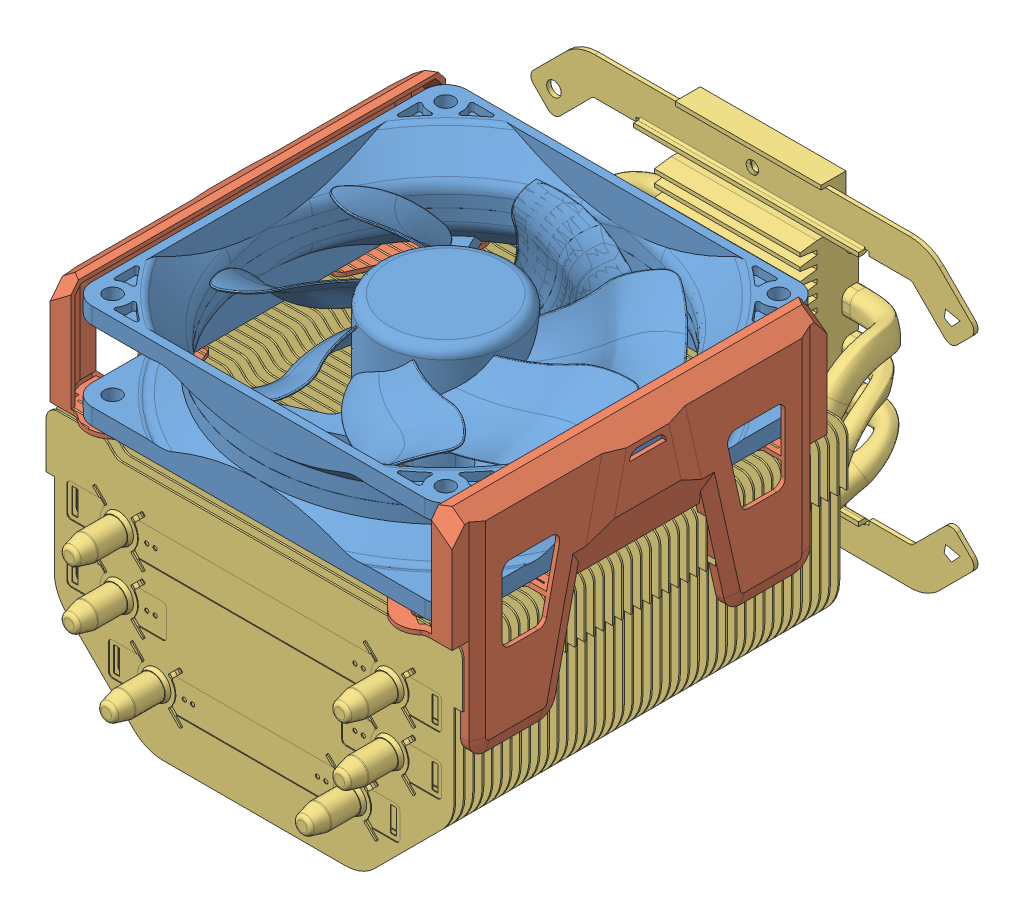
SolidWorks assembly dissipador, configuration Default. Lengths in mm.
Overall size (108.44 87.6 180.01).
4 component instances, 3 part files, 0 mates.
Components (placement in the parent):
- 7030025_PART_FAN STANDARD 90_MODEL.igs-1: 7030025_PART_FAN STANDARD 90_MODEL.igs [Default] at (0 45 -45) x (1 0 0) z (0 -1 0) size (93.98 180.01 25.07)
- 7030026_PART_HEATSINK ADAPTOR 90_MODEL.igs-1: 7030026_PART_HEATSINK ADAPTOR 90_MODEL.igs [Default] at (95 58.5 47.4641) x (0 0 -1) z (-1 0 0) size (106.39 52.6 26.58)
- 7030026_PART_HEATSINK ADAPTOR 90_MODEL.igs-2: 7030026_PART_HEATSINK ADAPTOR 90_MODEL.igs [Default] at (-7 58.5 -46) x (0 0 1) z (1 0 0) size (106.39 52.6 26.58)
- 7030027_PART_CPU HEATSINK TOWER_MODEL.igs-1: 7030027_PART_CPU HEATSINK TOWER_MODEL.igs [Default] at (94 31.5 -47.65) x (-1 0 0) z (0 0 1) size (108.44 80.01 139.76)
